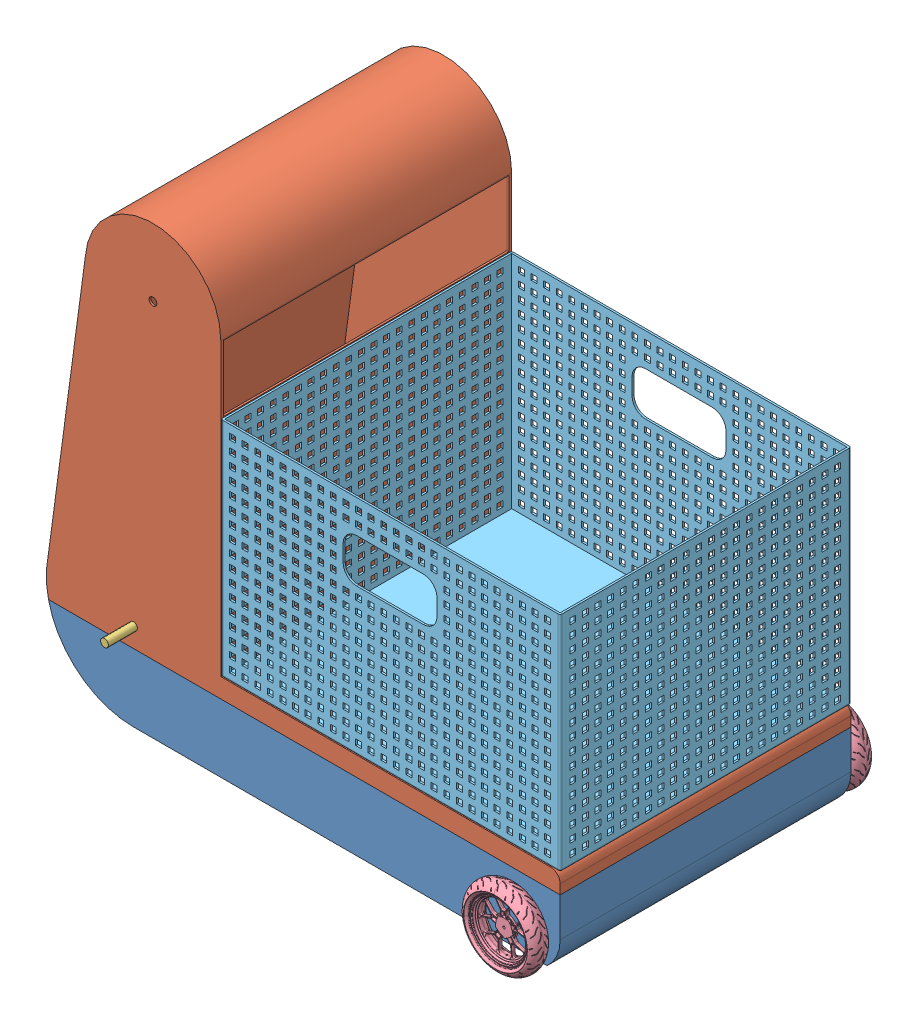
SolidWorks assembly Tennibot.6.0, configuration 默认. Lengths in mm.
Overall size (545.22 485.28 360).
8 component instances, 6 part files, 12 mates.
Components (placement in the parent):
- 底盘-1: 底盘 [默认] at (-167.8027 16.2482 527.7496) size (527.75 70 300)
- 上壳-1: 上壳 [默认] at (-167.8027 16.2482 527.7496) size (530 390 300)
- 轴_带轮1-1: 轴_带轮1 [默认] at (-167.8027 16.2482 197.7496) size (8 8 360)
- latter_wheel-1: latter_wheel [默认] at (232.2274 -43.7998 211.2059) x (-0.848125 -0.529796 0) z (0 0 -1) size (80 80.27 20.58)
- latter_wheel-2: latter_wheel [默认] at (232.2004 -43.8083 544.2934) x (0.998554 0.053749 0) z (0 0 1) size (80 80.27 20.58)
- front_wheel-3: front_wheel [默认] at (351.0415 -53.1737 917.1696) x (0.923728 0.383049 0) z (0 0 -1) size (200 200.68 51.45) (hidden)
- front_wheel-4: front_wheel [默认] at (467.1413 -66.8192 1125.6339) x (0.992599 -0.121438 0) z (0 0 1) size (200 200.68 51.45) (hidden)
- box-1: box [默认] at (97.1973 16.2482 377.7496) x (0 0 -1) z (0 1 0) size (300 350 230)
Mates (geometry in assembly coordinates):
- 重合1: coincident anti-aligned: plane of 底盘-1 through (-190.6419 -3.7518 227.7496) normal (0 1 0); plane of 上壳-1 through (232.1973 -3.7518 227.7496) normal (0 -1 0)
- 重合2: coincident aligned: plane of 底盘-1 through (232.1973 -43.7518 527.7496) normal (0 0 1); plane of 上壳-1 through (-147.8027 316.2482 527.7496) normal (0 0 1)
- 重合3: coincident aligned: plane of 底盘-1 through (272.1973 -43.7518 227.7496) normal (1 0 0); plane of 上壳-1 through (272.1973 -3.7518 227.7496) normal (1 0 0)
- 重合5: coincident aligned: plane of 轴_带轮1-1 through (-167.8027 16.2482 377.7496) normal (0 0 1)
- 同心2: concentric anti-aligned: cylinder of 上壳-1 through (-167.8027 16.2482 227.7496) axis (0 0 1) radius 4; cylinder of 轴_带轮1-1 through (-167.8027 16.2482 557.7496) axis (0 0 -1) radius 4
- 同心11: concentric aligned: cylinder of 底盘-1 through (232.1973 -43.7518 227.7496) axis (0 0 1) radius 4; cylinder of latter_wheel-1 through (232.1973 -43.7518 201.2609) axis (0 0 1) radius 1.2862
- 同心12: concentric anti-aligned: cylinder of 底盘-1 through (232.1973 -43.7518 227.7496) axis (0 0 1) radius 4; cylinder of latter_wheel-2 through (232.1973 -43.7518 554.2384) axis (0 0 -1) radius 1.2862
- 距离1: distance = 18 mm aligned: plane of latter_wheel-1 through (232.1973 -43.7518 209.7496) normal (0 0 -1); plane of 底盘-1 through (232.1973 -43.7518 227.7496) normal (0 0 -1)
- 距离2: distance = 18 mm aligned: plane of 底盘-1 through (232.1973 -43.7518 527.7496) normal (0 0 1); plane of latter_wheel-2 through (232.1973 -43.7518 545.7496) normal (0 0 1)
- 重合14: coincident anti-aligned: plane of 上壳-1 through (272.1973 16.2482 227.7496) normal (0 1 0); plane of box-1 through (97.1973 16.2482 377.7496) normal (0 -1 0)
- 重合16: coincident aligned: plane of 底盘-1 through (232.1973 -43.7518 527.7496) normal (0 0 1); plane of box-1 through (-77.8027 246.2482 527.7496) normal (0 0 1)
- 重合17: coincident aligned: plane of 底盘-1 through (272.1973 -43.7518 227.7496) normal (1 0 0); plane of box-1 through (272.1973 246.2482 227.7496) normal (1 0 0)
